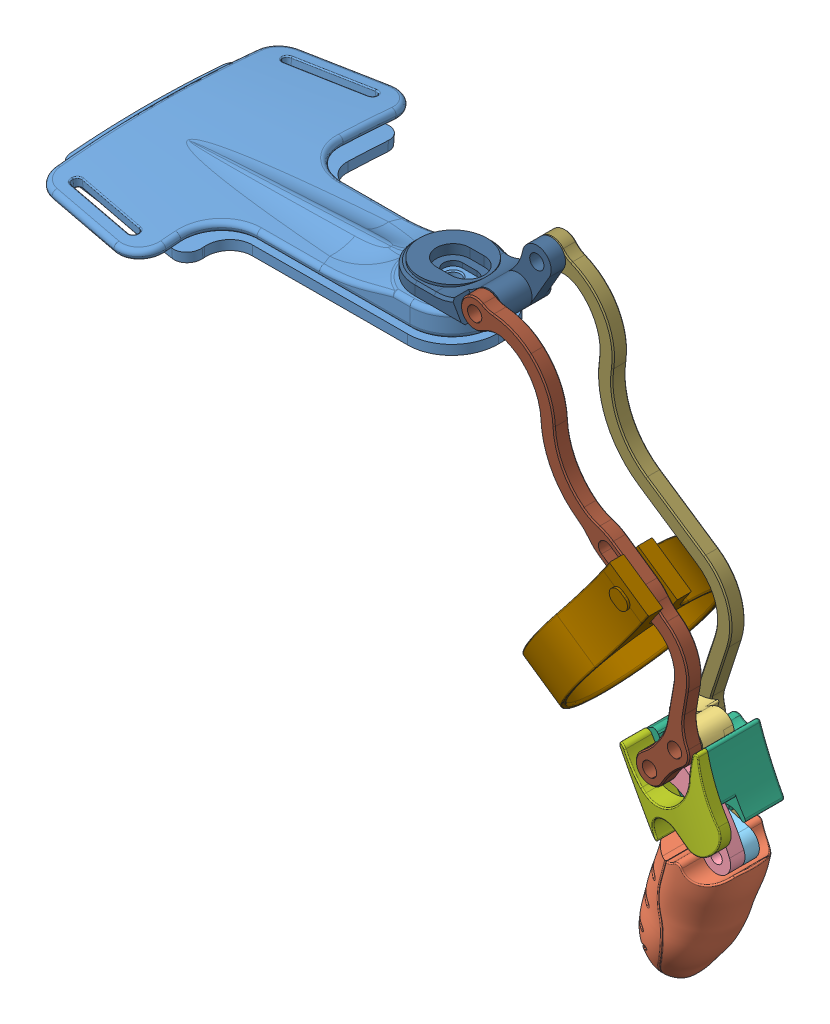
SolidWorks assembly Main assembly, configuration По умолчанию. Lengths in mm.
Overall size (141.3 118.46 58.61).
14 component instances, 13 part files, 14 mates.
Components (placement in the parent):
- Wrist plate-1: Wrist plate [По умолчанию] at origin
- Distal phalange-1: Distal phalange [По умолчанию] at (94.9303 -66.3773 4) x (0.265283 0.964171 0) z (0 0 -1)
- Mechanism-1: Mechanism [По умолчанию] at (86.4638 -51.8605 -1.5) x (0.406971 -0.913441 0) z (0 0 1) size (32.07 21.49 18.03) (flexible)
  - Main-1: Main [По умолчанию] at origin size (21 13.47 9)
  - Distal-1: Distal [По умолчанию] at (3.4326 0.7738 0) x (0.987405 -0.158211 0) z (0 0 1) size (20.35 13.53 3)
  - Link-1: Link [По умолчанию] at (2.9247 9.2259 0) x (0.772751 -0.63471 0) z (0 0 1) size (13 13 3)
  - Fairing with silicon pad-1: Fairing with silicon pad [По умолчанию] at origin size (18.09 19.19 13)
  - H-Fairing-1: H-Fairing [По умолчанию] at origin size (17.69 19.29 7.14)
  - Silicon pad-1: Silicon pad [По умолчанию] at origin size (13.32 11.97 9.89)
- New Ring New-1: New Ring New [По умолчанию] at (71.2064 -35.7162 3.5) x (0 0 -1) z (0.822776 -0.568366 0)
- Base new_v2-1: Base new_v2 [По умолчанию] at (40 6.5 4)
- Слепок руки v1-1: Слепок руки v1 [По умолчанию] at (-25.2805 -42.789 -6.643) x (-0.023219 0.948334 0.316424) z (0.998466 0.037912 -0.040357) (hidden)
- shatun 1 new-3: shatun 1 new [По умолчанию] at (38.9834 12.4272 8.5) x (0.901316 -0.433163 0) z (0 0 1)
- shatun 2 new-1: shatun 2 new [По умолчанию] at (86.8439 -51.8729 -0.5) x (-0.767853 0.640626 0) z (0 0 -1)
Mates (geometry in assembly coordinates):
- Hinge28: hinge anti-aligned: cylinder of Base new_v2-1 through (40 6 4) axis (0 1 0) radius 2; cylinder of Wrist plate-1 through (40 17.8137 4) axis (0 -1 0) radius 1.5; plane of Base new_v2-1 through (40 6.5 4) normal (0 -1 0); plane of Wrist plate-1 through (0 6.5 0) normal (0 1 0)
- Angle1: planar angle = 0 rad aligned: plane of Base new_v2-1 through (40 6.5 12) normal (0 0 1); plane of Wrist plate-1 through (0 -5 13) normal (0 0 1)
- Hinge29: hinge anti-aligned: cylinder of shatun 2 new-1 through (56 16.4282 -3.5) axis (0 0 -1) radius 1.25; cylinder of shatun 2 new-1 through (56 16.4282 -0.5) axis (0 0 -1) radius 1.5; plane of Base new_v2-1 through (81.1091 -32.6324 -0.5) normal (0 0 1); plane of Base new_v2-1 through (40 6.5 -0.5) normal (0 0 -1)
- Hinge31: hinge anti-aligned: cylinder of shatun 2 new-1 through (86.6806 -51.0483 -3.5) axis (0 0 -1) radius 1.25; cylinder of Mechanism-1/Main-1 through (86.6806 -51.0483 8.501) axis (0 0 -1) radius 1.25; plane of Mechanism-1/Main-1 through (86.4638 -51.8605 -0.5) normal (0 0 -1); plane of shatun 2 new-1 through (81.1091 -32.6324 -0.5) normal (0 0 1)
- Hinge32: hinge anti-aligned: cylinder of shatun 1 new-3 through (93.7713 -48.6047 11.5) axis (0 0 1) radius 1.5; cylinder of shatun 1 new-3 through (93.7713 -48.6047 8.5) axis (0 0 -1) radius 1.25; plane of Mechanism-1/Main-1 through (54.8037 -1.7755 8.5) normal (0 0 -1); plane of Mechanism-1/Main-1 through (86.4638 -51.8605 8.5) normal (0 0 1)
- Concentric4: concentric aligned: cylinder of Mechanism-1/Distal-1 through (88.5676 -54.681 -1.501) axis (0 0 1) radius 1.25; cylinder of shatun 1 new-3 through (88.5676 -54.681 11.5) axis (0 0 1) radius 1.5
- Slot1: slot anti-aligned: cylinder of New Ring New-1 through (85.9623 -24.0322 20.5) axis (0 0 -1) radius 1.5; plane of shatun 1 new-3 through (78.5275 -20.7194 8.5) normal (0.568366 0.822776 0); cylinder of New Ring New-1 through (85.1395 -23.4638 20.5) axis (0 0 -1) radius 1.5; cylinder of shatun 1 new-3 through (85.9623 -24.0322 8.5) axis (0 0 1) radius 1.5
- Parallel2: parallel aligned: plane of New Ring New-1 through (83.1421 -18.4379 3.5) normal (0.568366 0.822776 0); plane of shatun 1 new-3 through (77.1938 -14.9365 11.5) normal (0.568366 0.822776 0)
- Coincident39: coincident anti-aligned: plane of Distal phalange-1 through (92.5427 -75.0548 4) normal (0.265283 0.964171 0); plane of Mechanism-1/Link-1 through (96.3994 -76.1159 13.5623) normal (-0.265283 -0.964171 0)
- Coincident40: coincident anti-aligned: plane of Distal phalange-1 through (92.5427 -75.0548 5.5) normal (0 0 -1); plane of Mechanism-1/Link-1 through (96.0813 -50.7774 5.5) normal (0 0 1)
- Concentric5: concentric anti-aligned: cylinder of New Ring New-1 through (85.9623 -24.0322 20.5) axis (0 0 -1) radius 1.5; cylinder of shatun 1 new-3 through (85.9623 -24.0322 8.5) axis (0 0 1) radius 1.5
- Hinge33: hinge anti-aligned: cylinder of shatun 1 new-3 through (52 9.5 11.5) axis (0 0 1) radius 1.5; cylinder of Base new_v2-1 through (52 9.5 -4) axis (0 0 1) radius 1.5; plane of shatun 1 new-3 through (54.8037 -1.7755 8.5) normal (0 0 -1); plane of Base new_v2-1 through (40 6.5 8.5) normal (0 0 1)
- Coincident42: coincident anti-aligned: plane of New Ring New-1 through (71.2064 -35.7162 11.5) normal (0 0 -1); plane of shatun 1 new-3 through (54.8037 -1.7755 11.5) normal (0 0 1)
- Distance1: distance = 0 mm anti-aligned: plane of Distal phalange-1 through (96.3994 -76.1159 5.5) normal (-0.964171 0.265283 0); plane of Mechanism-1/Link-1 through (98.2564 -69.3667 13.5623) normal (0.964171 -0.265283 0)
